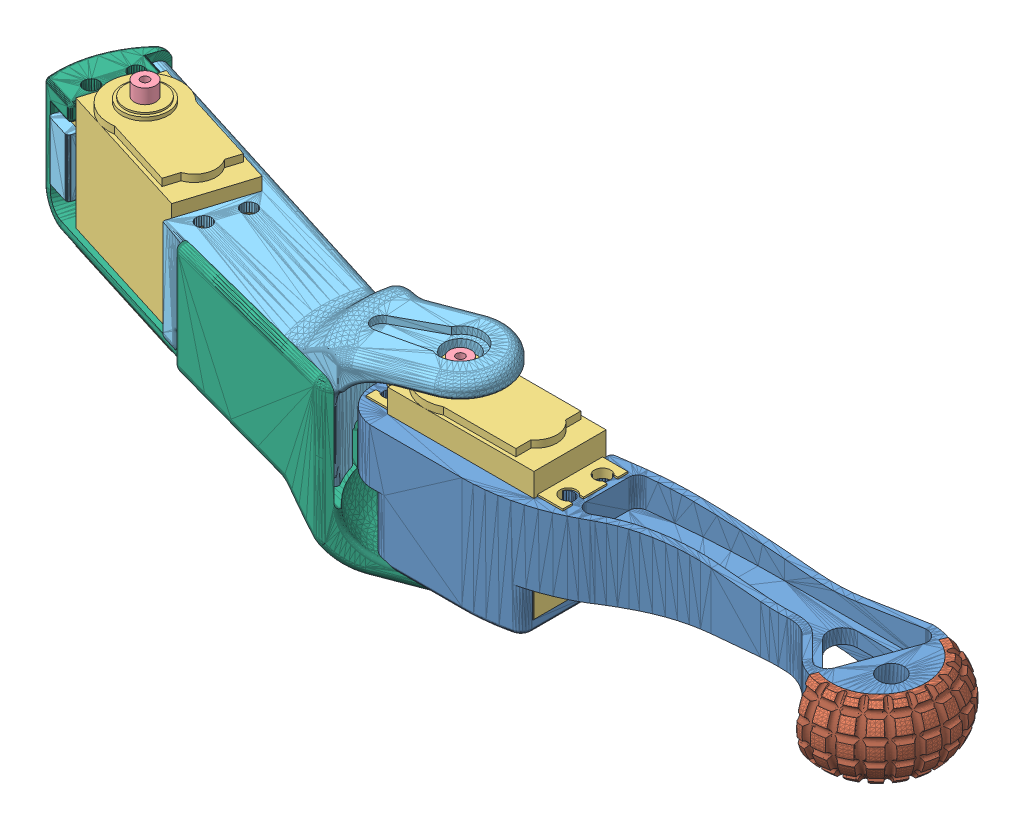
SolidWorks assembly Assem1, configuration Default. Lengths in mm.
Overall size (273.19 54.9 82.13).
10 component instances, 6 part files, 17 mates.
Components (placement in the parent):
- L_wrist_mg-1: L_wrist_mg [Default] at (-104.9134 49.2874 139.9903) size (149.99 36.9 30)
- foot-1: foot [Default] at (21.0866 19.2874 149.9903) x (0.342019 0 -0.939693) z (-0.939693 0 -0.342019) size (38.32 20 19.41)
- MG996R-1: MG996R [Default] at (-84.6634 -9.7126 149.9903) size (54.5 43 20)
  - servo-1: servo [Default] at origin size (54.5 39 20)
  - shaft-1: shaft [Default] at (-10.1089 43 0) x (-0.837169 0 -0.546944) z (-0.546944 0 0.837169) size (5.9 19.57 5.9)
- L_arm_mg-1: L_arm_mg [Default] at (-207.5148 26.2874 118.7288) x (-0.298458 0 0.954423) z (0.954423 0 0.298458) size (38.24 39.8 137.4)
- MG996R-2: MG996R [Default] at (-191.1723 -5.7126 134.3168) x (0.954423 0 0.298458) z (-0.298458 0 0.954423) size (54.5 43 20)
  - servo-1: servo [Default] at origin size (54.5 39 20)
  - shaft-1: shaft [Default] at (-10.1089 43 0) x (-0.837169 0 -0.546944) z (-0.546944 0 0.837169) size (5.9 19.57 5.9)
- L_arm_cover-1: L_arm_cover [Default] at (-212.5542 28.5874 111.3903) x (-0.298458 0 0.954423) z (0.954423 0 0.298458) size (41.16 45 143.55)
Mates (geometry in assembly coordinates):
- Coincident1: coincident anti-aligned: plane of L_wrist_mg-1 through (9.5615 49.2874 181.6556) normal (0.939693 0 0.342019); plane of foot-1 through (21.0866 19.2874 149.9903) normal (-0.939693 0 -0.342019)
- Parallel2: parallel aligned: line of foot-1 through (16.6404 -0.7126 162.2063) axis (0 1 0); line of L_wrist_mg-1 through (16.6404 -0.7126 162.2063) axis (0 1 0)
- Coincident4: coincident: point of foot-1; point of L_wrist_mg-1
- Coincident5: coincident anti-aligned: plane of L_wrist_mg-1 through (-104.9134 49.2874 159.9903) normal (0 0 -1); plane of MG996R-1/servo-1 through (-104.9134 25.7874 159.9903) normal (0 0 1)
- Coincident6: coincident anti-aligned: plane of L_wrist_mg-1 through (-104.9134 -9.7126 139.9903) normal (0 1 0); plane of MG996R-1/servo-1 through (-84.6634 -9.7126 149.9903) normal (0 -1 0)
- Coincident7: coincident anti-aligned: plane of L_wrist_mg-1 through (-64.4134 49.2874 139.9903) normal (-1 0 0); plane of MG996R-1/servo-1 through (-64.4134 25.7874 159.9903) normal (1 0 0)
- Parallel4: parallel aligned: plane of MG996R-1/servo-1 through (-94.7723 27.7874 149.9903) normal (0 1 0); plane of L_arm_mg-1 through (-207.5148 26.2874 118.7288) normal (0 1 0)
- Coincident14: coincident anti-aligned: plane of L_arm_mg-1 through (-207.5148 21.2874 118.7288) normal (0 1 0); plane of MG996R-2/servo-1 through (-213.138 21.2874 122.4711) normal (0 -1 0)
- Coincident15: coincident anti-aligned: plane of L_arm_mg-1 through (-207.5148 26.2874 118.7288) normal (0.954423 0 0.298458); plane of MG996R-2/servo-1 through (-213.484 29.7874 137.8173) normal (-0.954423 0 -0.298458)
- Coincident16: coincident anti-aligned: plane of L_arm_mg-1 through (-207.5148 26.2874 118.7288) normal (-0.298458 0 0.954423); plane of MG996R-2/servo-1 through (-207.5148 29.7874 118.7288) normal (0.298458 0 -0.954423)
- Coincident18: coincident: line of MG996R-1/shaft-1 through (-94.7723 33.2874 149.9903) axis (0 -1 0)
- Distance1: distance = 2 mm: line of L_arm_mg-1 through (-92.2047 31.2874 153.6718) axis (-0.572046 0 -0.820221)
- Coincident21: coincident anti-aligned: plane of L_arm_cover-1 through (-212.5542 23.7874 111.3903) normal (0 -1 0); plane of MG996R-2/servo-1 through (-213.138 23.7874 122.4711) normal (0 1 0)
- Parallel5: parallel anti-aligned: plane of MG996R-2/servo-1 through (-213.484 29.7874 137.8173) normal (-0.954423 0 -0.298458); plane of L_arm_cover-1 through (-205.8733 28.5874 113.4795) normal (0.954423 0 0.298458)
- Coincident23: coincident anti-aligned: plane of MG996R-2/servo-1 through (-213.484 29.7874 137.8173) normal (-0.954423 0 -0.298458); plane of L_arm_cover-1 through (-205.8733 28.5874 113.4795) normal (0.954423 0 0.298458)
- Parallel6: parallel aligned: plane of L_arm_mg-1 through (-206.0225 26.2874 113.9567) normal (0.298458 0 -0.954423); plane of L_arm_cover-1 through (-212.5542 28.5874 111.3903) normal (0.298458 0 -0.954423)
- Coincident25: coincident anti-aligned: plane of L_arm_mg-1 through (-207.5148 26.2874 118.7288) normal (-0.298458 0 0.954423); plane of L_arm_cover-1 through (-214.1958 28.5874 116.6396) normal (0.298458 0 -0.954423)
